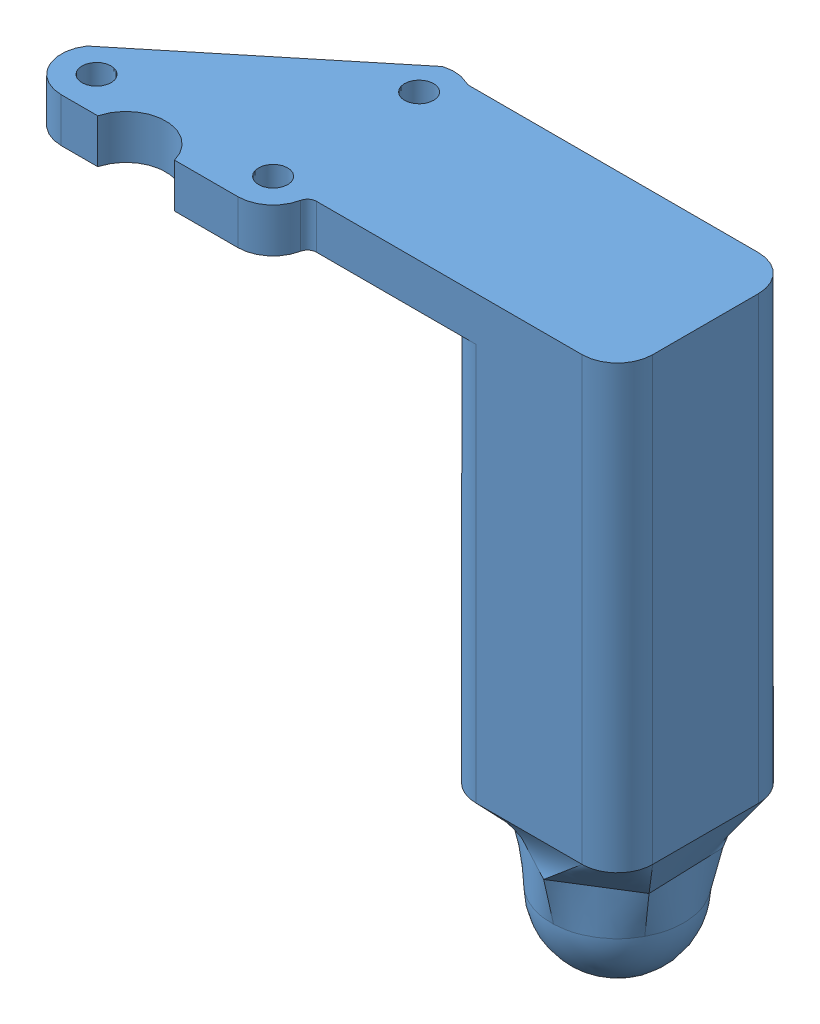
SolidWorks assembly shock_absorber, configuration Default. Lengths in mm.
Overall size (75.17 67.5 68.6).
2 component instances, 2 part files, 0 mates.
Components (placement in the parent):
- landing-1: landing [Default] at (-64.8969 55.0277 16.1188) x (0.848048 0 -0.529919) z (0.529919 0 0.848048) size (62.5 67.5 41.84)
- shaft-1: shaft [Default] at (-27.9284 17.5277 9.3678) size (2.9 2.9 7)
